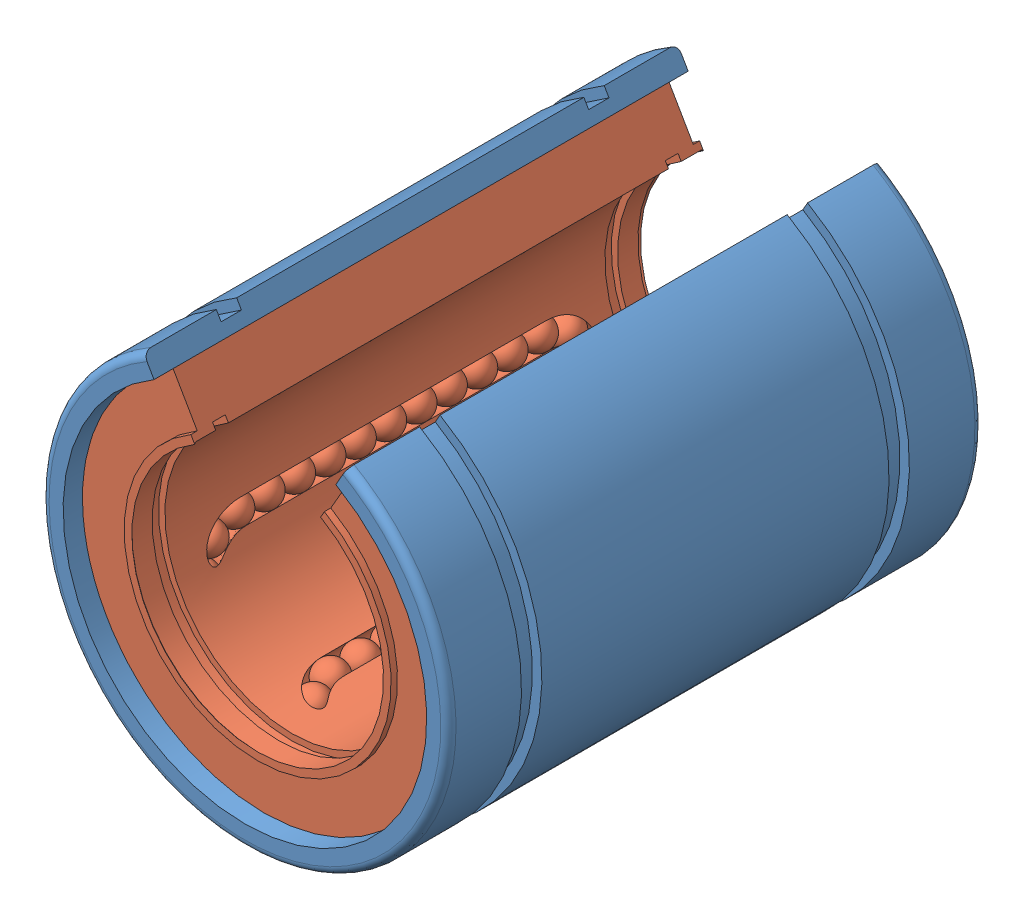
SolidWorks assembly LM20OP, configuration Default. Lengths in mm.
Overall size (39.07 39.07 42.07).
2 component instances, 2 part files, 2 mates.
Components (placement in the parent):
- LM20OP-1-2: LM20OP-1 [Default] at (-2.5166 3.2076 -21.2217) size (32 29.9 42.07)
- LM20OP-2-2: LM20OP-2 [Default] at (4.6334 15.5917 -0.2217) x (0 0 -1) z (-0.5 -0.866025 0) size (40 28.6 28.6)
Mates (geometry in assembly coordinates):
- Coincident9: coincident: moEndPointRef_w of LM20OP-1-2; moEndPointRef_w of LM20OP-2-2
- Concentric4: concentric anti-aligned: cylinder of LM20OP-1-2 through (-2.5166 3.2076 20.7783) axis (0 0 -1) radius 14.3; cylinder of LM20OP-2-2 through (-2.5166 3.2076 19.7783) axis (0 0 1) radius 14.3
